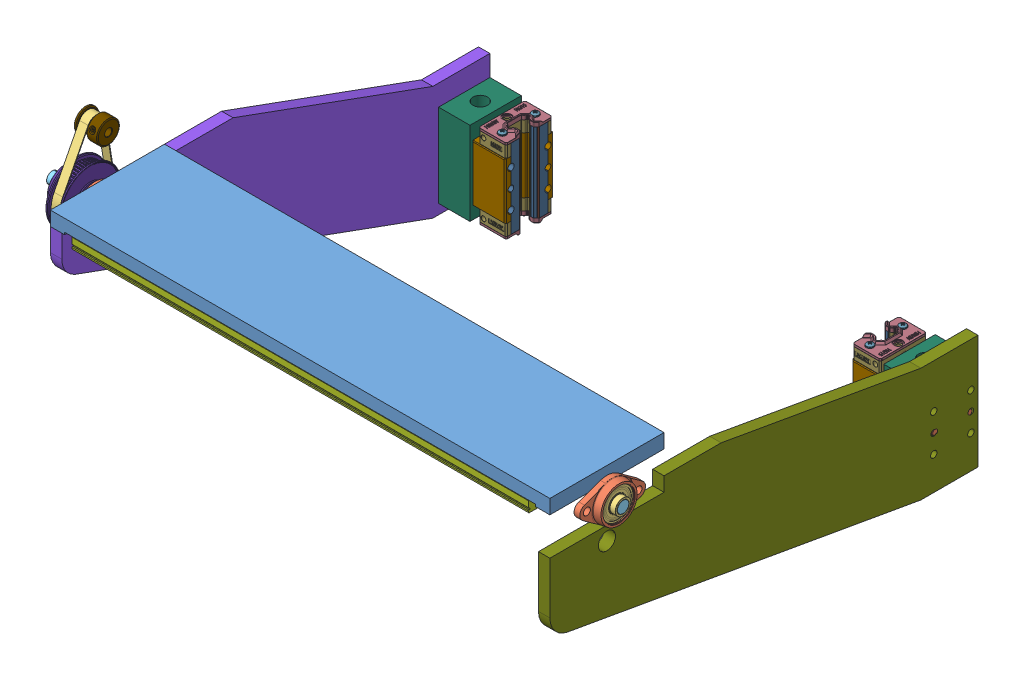
SolidWorks assembly Eje_X, configuration Predeterminado. Lengths in mm.
Overall size (400 162.38 300).
52 component instances, 22 part files, 43 mates.
Components (placement in the parent):
- Puente_X^Eje_X-1: Puente_X^Eje_X [Predeterminado] at (-189.2038 15.372 -72.2278) x (1 0 0) z (0 -1 0) size (350 80 10) (virtual)
- KFL08-1: KFL08 [Varsayılan] at (-189.2038 -4.128 -32.2278) x (0 -0.043192 0.999067) z (0 -0.999067 -0.043192) size (46.5 11.35 27)
  - FLANGE-1: FLANGE [Default] at origin size (46.5 8.5 27)
  - BEARING-1: BEARING [Default] at (0 4 0) x (1 0 0) z (0 -1 0) size (22 22 10.85)
  - socket set screw cone point_am-1: socket set screw cone point_am [B18.3.6M - M2.5 x 0.45 x 2 Hex Socket Cone Pt. SS --S] at (0 9.425 5.45) x (0 0 -1) z (1 0 0) size (2 2.5 2.5)
  - socket set screw cone point_am-2: socket set screw cone point_am [B18.3.6M - M2.5 x 0.45 x 2 Hex Socket Cone Pt. SS --S] at (5.45 9.425 0) x (-1 0 0) z (0 0 -1) size (2 2.5 2.5)
- ax_Y_LeadScrew_Nut_8mm_x_2mmPitch-1: ax_Y_LeadScrew_Nut_8mm_x_2mmPitch [Default] at (-227.8538 -4.128 -32.2278) x (0 0.538804 0.842431) z (-1 0 0) size (8 8 400)
- eje_X_guia_inf-1: eje_X_guia_inf [Predeterminado] at (75.7962 2.9226 -66.2278) x (0 0 -1) z (-1 0 0) size (12 8.1 320)
- eje_X_guia_sup-1: eje_X_guia_sup [Predeterminado] at (-104.2038 2.9226 1.7722) x (0 0 1) z (1 0 0) size (12 8.1 320)
-  Columa_xn^Eje_X-1:  Columa_xn^Eje_X [Predeterminado] at (-181.2038 -35.5839 -292.2278) x (0 -1 0) z (-1 0 0) size (130.96 300 8) (virtual)
- HGH15CA-1: HGH15CA [Default] at (-131.2038 -79.3839 -274.2278) x (0 0 -1) z (0 1 0) size (34 23.7 61.49)
  - HGH15CA Block-1: HGH15CA Block [HGR15R300CE20] at origin size (34 23.7 39.4)
  - HGx15CA Retainer-1: HGx15CA Retainer [HGR15R300CE20] at origin size (26 4 55.4)
  - HGx15CA Tiny Red-1: HGx15CA Tiny Red [HGR15R300CE20] at origin size (14.2 1 55.4)
  - HGx15CA End Cap-1: HGx15CA End Cap [HGR15R300CE20] at origin size (32.5 19.5 8)
  - HGx15CA End Cap-2: HGx15CA End Cap [HGR15R300CE20] x (-1 0 0) z (0 0 -1) size (32.5 19.5 8)
  - HGx15CA Seal-1: HGx15CA Seal [HGR15R300CE20] at origin size (32.5 19.5 3)
  - HGx15CA Seal-2: HGx15CA Seal [HGR15R300CE20] x (-1 0 0) z (0 0 -1) size (32.5 19.5 3)
  - pan head cross recess screw_iso-1: pan head cross recess screw_iso [ISO 7045 - M2.5 x 16 - Z - 16C] at (11.5 11.8 30.8) x (0 0 -1) z (0 -1 0) size (18.05 5 5)
  - pan head cross recess screw_iso-2: pan head cross recess screw_iso [ISO 7045 - M2.5 x 16 - Z - 16C] at (-11.5 11.8 30.8) x (0 0 -1) z (0 1 0) size (18.05 5 5)
  - pan head cross recess screw_iso-3: pan head cross recess screw_iso [ISO 7045 - M2.5 x 16 - Z - 16C] at (11.5 11.8 -30.8) x (0 0 1) z (0 -1 0) size (18.05 5 5)
  - pan head cross recess screw_iso-4: pan head cross recess screw_iso [ISO 7045 - M2.5 x 16 - Z - 16C] at (-11.5 11.8 -30.8) x (0 0 1) z (0 1 0) size (18.05 5 5)
- Soporte_tuerca_husillo_X^Eje_X-1: Soporte_tuerca_husillo_X^Eje_X [Predeterminado] at (-159.2038 -108.5839 -256.2278) x (0 1 0) z (-1 0 0) size (58.4 36 22) (virtual)
- Columa_xp^Eje_X-1: Columa_xp^Eje_X [Predeterminado] at (160.7962 -35.5839 -292.2278) x (0 -1 0) z (-1 0 0) size (130.96 300 8) (virtual)
- HGH15CA-2: HGH15CA [Default] at (102.7962 -79.3839 -274.2278) x (0 0 -1) z (0 -1 0) size (34 23.7 61.49)
  - HGH15CA Block-1: HGH15CA Block [HGR15R300CE20] at origin size (34 23.7 39.4)
  - HGx15CA Retainer-1: HGx15CA Retainer [HGR15R300CE20] at origin size (26 4 55.4)
  - HGx15CA Tiny Red-1: HGx15CA Tiny Red [HGR15R300CE20] at origin size (14.2 1 55.4)
  - HGx15CA End Cap-1: HGx15CA End Cap [HGR15R300CE20] at origin size (32.5 19.5 8)
  - HGx15CA End Cap-2: HGx15CA End Cap [HGR15R300CE20] x (-1 0 0) z (0 0 -1) size (32.5 19.5 8)
  - HGx15CA Seal-1: HGx15CA Seal [HGR15R300CE20] at origin size (32.5 19.5 3)
  - HGx15CA Seal-2: HGx15CA Seal [HGR15R300CE20] x (-1 0 0) z (0 0 -1) size (32.5 19.5 3)
  - pan head cross recess screw_iso-1: pan head cross recess screw_iso [ISO 7045 - M2.5 x 16 - Z - 16C] at (11.5 11.8 30.8) x (0 0 -1) z (0 -1 0) size (18.05 5 5)
  - pan head cross recess screw_iso-2: pan head cross recess screw_iso [ISO 7045 - M2.5 x 16 - Z - 16C] at (-11.5 11.8 30.8) x (0 0 -1) z (0 1 0) size (18.05 5 5)
  - pan head cross recess screw_iso-3: pan head cross recess screw_iso [ISO 7045 - M2.5 x 16 - Z - 16C] at (11.5 11.8 -30.8) x (0 0 1) z (0 -1 0) size (18.05 5 5)
  - pan head cross recess screw_iso-4: pan head cross recess screw_iso [ISO 7045 - M2.5 x 16 - Z - 16C] at (-11.5 11.8 -30.8) x (0 0 1) z (0 1 0) size (18.05 5 5)
- Soporte_tuerca_husillo_X^Eje_X-2: Soporte_tuerca_husillo_X^Eje_X [Predeterminado] at (130.7962 -50.1839 -256.2278) x (0 -1 0) z (1 0 0) size (58.4 36 22) (virtual)
- KFL08-2: KFL08 [Varsayılan] at (160.7962 -4.128 -32.2278) x (0 -0.14239 -0.989811) z (0 -0.989811 0.14239) size (46.5 11.35 27)
  - FLANGE-1: FLANGE [Default] at origin size (46.5 8.5 27)
  - BEARING-1: BEARING [Default] at (0 4 0) x (1 0 0) z (0 -1 0) size (22 22 10.85)
  - socket set screw cone point_am-1: socket set screw cone point_am [B18.3.6M - M2.5 x 0.45 x 2 Hex Socket Cone Pt. SS --S] at (0 9.425 5.45) x (0 0 -1) z (1 0 0) size (2 2.5 2.5)
  - socket set screw cone point_am-2: socket set screw cone point_am [B18.3.6M - M2.5 x 0.45 x 2 Hex Socket Cone Pt. SS --S] at (5.45 9.425 0) x (-1 0 0) z (0 0 -1) size (2 2.5 2.5)
- Copia de GT2_60T_8_6^Eje_X-1: Copia de GT2_60T_8_6^Eje_X [Default] at (-211.3538 -4.128 -32.2278) x (0 -0.85392 -0.520404) z (1 0 0) size (42 42 18) (virtual)
- Copia de GT2_20T^Eje_X-1: Copia de GT2_20T^Eje_X [Конфигурация1] at (-194.9038 36.3557 -38.7137) x (-1 0 0) z (0 0.380598 0.924741) size (16 16 16) (virtual)
- Copia de NEMA 23HS7430^Eje_X-1: Copia de NEMA 23HS7430^Eje_X [По умолчанию] at (-187.6038 45.572 -50.4278) x (0 1 0) z (1 0 0) size (58.4 56.4 95.6) (hidden, virtual)
- Copia de T8_nut^Eje_X-1: Copia de T8_nut^Eje_X [Default] at (-170.2038 -112.5839 -274.4641) x (0.063591 0 0.997976) z (-0.997976 0 0.063591) size (22.03 15.25 22.03) (virtual)
- Copia de T8_nut^Eje_X-2: Copia de T8_nut^Eje_X [Default] at (141.7962 -112.5839 -274.4641) x (0.864495 0 0.502641) z (-0.502641 0 0.864495) size (22.03 15.25 22.03) (virtual)
- guia_4x20^Eje_X-1: guia_4x20^Eje_X [Predeterminado] at (-169.2038 -79.3839 -262.2278) x (0 0 1) z (-1 0 0) size (4 4 20) (virtual)
- guia_4x20^Eje_X-2: guia_4x20^Eje_X [Predeterminado] at (-169.2038 -79.3839 -286.2278) x (0 0 1) z (-1 0 0) size (4 4 20) (virtual)
- Correa_158^Eje_X-1: Correa_158^Eje_X [Predeterminado] at (-209.3538 -4.128 -32.2278) x (0 0.987408 -0.158192) z (1 0 0) size (66.95 38.7 6) (virtual)
- guia_4x20^Eje_X-3: guia_4x20^Eje_X [Predeterminado] at (140.7962 -79.3839 -262.2278) x (0 -0.924225 -0.381849) z (1 0 0) size (4 4 20) (virtual)
- guia_4x20^Eje_X-4: guia_4x20^Eje_X [Predeterminado] at (140.7962 -79.3839 -286.2278) x (0 -0.305624 0.952152) z (1 0 0) size (4 4 20) (virtual)
Mates (geometry in assembly coordinates):
- Coincidente8: coincident aligned: plane of Puente_X^Eje_X-1 through (-189.2038 5.372 7.7722) normal (-1 0 0); plane of  Columa_xn^Eje_X-1 through (-189.2038 -10.4485 -7.2278) normal (-1 0 0)
- Coincidente9: coincident anti-aligned: plane of Puente_X^Eje_X-1 through (-189.2038 5.372 -72.2278) normal (0 -1 0); plane of  Columa_xn^Eje_X-1 through (-189.2038 5.372 7.7722) normal (0 1 0)
- Coincidente10: coincident anti-aligned: plane of Puente_X^Eje_X-1 through (160.7962 5.372 -72.2278) normal (0 0 -1); plane of  Columa_xn^Eje_X-1 through (-189.2038 15.372 -72.2278) normal (0 0 1)
- Coincidente11: coincident aligned: plane of Puente_X^Eje_X-1 through (160.7962 5.372 7.7722) normal (1 0 0); plane of Columa_xp^Eje_X-1 through (160.7962 -10.4485 -7.2278) normal (1 0 0)
- Coincidente12: coincident anti-aligned: plane of Puente_X^Eje_X-1 through (160.7962 5.372 -72.2278) normal (0 0 -1); plane of Columa_xp^Eje_X-1 through (152.7962 15.372 -72.2278) normal (0 0 1)
- Coincidente13: coincident anti-aligned: plane of Puente_X^Eje_X-1 through (-189.2038 5.372 -72.2278) normal (0 -1 0); plane of Columa_xp^Eje_X-1 through (152.7962 5.372 7.7722) normal (0 1 0)
- Coincidente16: coincident aligned: plane of Puente_X^Eje_X-1 through (160.7962 5.372 7.7722) normal (0 0 1); plane of eje_X_guia_sup-1 through (145.7962 6.872 7.7722) normal (0 0 1)
- Coincidente20: coincident anti-aligned: plane of KFL08-1/FLANGE-1 through (-189.2038 -4.9163 -13.9949) normal (1 0 0); plane of  Columa_xn^Eje_X-1 through (-189.2038 -10.4485 -7.2278) normal (-1 0 0)
- Concéntrica2: concentric anti-aligned: cylinder of KFL08-1/BEARING-1 through (-189.7038 -4.128 -32.2278) axis (1 0 0) radius 4; cylinder of ax_Y_LeadScrew_Nut_8mm_x_2mmPitch-1 through (172.1462 -4.128 -32.2278) axis (-1 0 0) radius 4
- Coincidente28: coincident anti-aligned: plane of Columa_xp^Eje_X-1 through (160.7962 -10.4485 -7.2278) normal (1 0 0); plane of KFL08-2/FLANGE-1 through (160.7962 -6.7267 -50.2919) normal (-1 0 0)
- Concéntrica3: concentric aligned: cylinder of ax_Y_LeadScrew_Nut_8mm_x_2mmPitch-1 through (172.1462 -4.128 -32.2278) axis (-1 0 0) radius 4; cylinder of KFL08-2/BEARING-1 through (161.2962 -4.128 -32.2278) axis (-1 0 0) radius 4
- Coincidente29: coincident aligned: plane of ax_Y_LeadScrew_Nut_8mm_x_2mmPitch-1 through (172.1462 -4.128 -32.2278) normal (1 0 0); plane of KFL08-2/BEARING-1 through (172.1462 -8.3842 -31.6155) normal (1 0 0)
- Concéntrica4: concentric aligned: cylinder of ax_Y_LeadScrew_Nut_8mm_x_2mmPitch-1 through (172.1462 -4.128 -32.2278) axis (-1 0 0) radius 4; cylinder of Copia de GT2_60T_8_6^Eje_X-1 through (-181.3538 -4.128 -32.2278) axis (-1 0 0) radius 4
- Distancia3: distance = 9 mm aligned: plane of Copia de GT2_60T_8_6^Eje_X-1 through (-218.8538 -4.128 -32.2278) normal (-1 0 0); plane of ax_Y_LeadScrew_Nut_8mm_x_2mmPitch-1 through (-227.8538 -4.128 -32.2278) normal (-1 0 0)
- Coincidente32: coincident aligned: plane of Puente_X^Eje_X-1 through (160.7962 5.372 -72.2278) normal (0 0 -1); plane of eje_X_guia_inf-1 through (-174.2038 6.872 -72.2278) normal (0 0 -1)
- Concéntrica6: concentric anti-aligned: cylinder of ax_Y_LeadScrew_Nut_8mm_x_2mmPitch-1 through (172.1462 -4.128 -32.2278) axis (-1 0 0) radius 4; cylinder of  Columa_xn^Eje_X-1 through (-189.2038 -4.128 -32.2278) axis (1 0 0) radius 6
- Coincidente33: coincident aligned: plane of Puente_X^Eje_X-1 through (-189.2038 5.372 7.7722) normal (-1 0 0); plane of Copia de NEMA 23HS7430^Eje_X-1 through (-189.2038 45.572 -50.4278) normal (-1 0 0)
- Distancia6: distance = 2 mm anti-aligned: plane of Copia de NEMA 23HS7430^Eje_X-1 through (-177.6038 17.372 -78.6278) normal (0 -1 0); plane of Puente_X^Eje_X-1 through (-189.2038 15.372 -72.2278) normal (0 1 0)
- Distancia7: distance = 30 mm aligned: plane of Copia de NEMA 23HS7430^Eje_X-1 through (-177.6038 17.372 -22.2278) normal (0 0 1); plane of Puente_X^Eje_X-1 through (160.7962 5.372 7.7722) normal (0 0 1)
- Coincidente42: coincident anti-aligned: plane of  Columa_xn^Eje_X-1 through (-181.2038 -10.4485 -7.2278) normal (1 0 0); plane of Soporte_tuerca_husillo_X^Eje_X-1 through (-181.2038 -108.5839 -256.2278) normal (-1 0 0)
- Distancia10: distance = 7 mm aligned: plane of Soporte_tuerca_husillo_X^Eje_X-1 through (-181.2038 -108.5839 -256.2278) normal (0 -1 0); plane of  Columa_xn^Eje_X-1 through (-189.2038 -115.5839 -292.2278) normal (0 -1 0)
- Coincidente44: coincident aligned: plane of  Columa_xn^Eje_X-1 through (-189.2038 -35.5839 -292.2278) normal (0 0 -1); plane of Soporte_tuerca_husillo_X^Eje_X-1 through (-181.2038 -108.5839 -292.2278) normal (0 0 -1)
- Coincidente45: coincident anti-aligned: plane of HGH15CA-1/HGH15CA Block-1 through (-159.2038 -59.6839 -290.2278) normal (-1 0 0); plane of Soporte_tuerca_husillo_X^Eje_X-1 through (-159.2038 -108.5839 -256.2278) normal (1 0 0)
- Distancia11: distance = 1 mm aligned: plane of HGH15CA-1/HGH15CA Block-1 through (-136.5038 -59.6839 -291.2278) normal (0 0 -1); plane of Soporte_tuerca_husillo_X^Eje_X-1 through (-181.2038 -108.5839 -292.2278) normal (0 0 -1)
- Coincidente47: coincident aligned: plane of HGH15CA-1/HGx15CA Seal-2 through (-137.6195 -108.5839 -279.3778) normal (0 -1 0); plane of Soporte_tuerca_husillo_X^Eje_X-1 through (-181.2038 -108.5839 -256.2278) normal (0 -1 0)
- Concéntrica7: concentric anti-aligned: cylinder of  Columa_xn^Eje_X-1 through (-189.2038 -79.3839 -262.2278) axis (-1 0 0) radius 2; cylinder of guia_4x20^Eje_X-1 through (-189.2038 -79.3839 -262.2278) axis (1 0 0) radius 2
- Coincidente48: coincident aligned: plane of  Columa_xn^Eje_X-1 through (-189.2038 -10.4485 -7.2278) normal (-1 0 0); plane of guia_4x20^Eje_X-1 through (-189.2038 -79.3839 -262.2278) normal (-1 0 0)
- Coincidente49: coincident aligned: plane of  Columa_xn^Eje_X-1 through (-189.2038 -10.4485 -7.2278) normal (-1 0 0); plane of guia_4x20^Eje_X-2 through (-189.2038 -79.3839 -286.2278) normal (-1 0 0)
- Concéntrica8: concentric anti-aligned: cylinder of  Columa_xn^Eje_X-1 through (-189.2038 -79.3839 -286.2278) axis (-1 0 0) radius 2; cylinder of guia_4x20^Eje_X-2 through (-189.2038 -79.3839 -286.2278) axis (1 0 0) radius 2
- Concéntrica9: concentric anti-aligned: cylinder of Correa_158^Eje_X-1 through (-203.3538 -4.128 -32.2278) axis (-1 0 0) radius 18.85; cylinder of Copia de GT2_60T_8_6^Eje_X-1 through (-218.8538 -4.128 -32.2278) axis (1 0 0) radius 12.5
- Distancia12: distance = 1 mm anti-aligned: plane of Correa_158^Eje_X-1 through (-203.3538 -4.128 -32.2278) normal (1 0 0); plane of Copia de GT2_60T_8_6^Eje_X-1 through (-202.3538 -4.128 -32.2278) normal (-1 0 0)
- Concéntrica10: concentric anti-aligned: cylinder of Copia de GT2_20T^Eje_X-1 through (-194.9038 36.3557 -38.7137) axis (1 0 0) radius 8; cylinder of Correa_158^Eje_X-1 through (-203.3538 36.3557 -38.7137) axis (-1 0 0) radius 6.1
- Distancia13: distance = 1 mm anti-aligned: plane of Correa_158^Eje_X-1 through (-203.3538 -4.128 -32.2278) normal (1 0 0); plane of Copia de GT2_20T^Eje_X-1 through (-202.3538 36.3557 -38.7137) normal (-1 0 0)
- Coincidente50: coincident anti-aligned: plane of Columa_xp^Eje_X-1 through (152.7962 -10.4485 -7.2278) normal (-1 0 0); plane of Soporte_tuerca_husillo_X^Eje_X-2 through (152.7962 -50.1839 -256.2278) normal (1 0 0)
- Coincidente51: coincident aligned: plane of Columa_xp^Eje_X-1 through (152.7962 -35.5839 -292.2278) normal (0 0 -1); plane of Soporte_tuerca_husillo_X^Eje_X-2 through (152.7962 -50.1839 -292.2278) normal (0 0 -1)
- Distancia14: distance = 7 mm aligned: plane of Soporte_tuerca_husillo_X^Eje_X-2 through (152.7962 -108.5839 -256.2278) normal (0 -1 0); plane of Columa_xp^Eje_X-1 through (152.7962 -115.5839 -292.2278) normal (0 -1 0)
- Coincidente53: coincident anti-aligned: circle of Soporte_tuerca_husillo_X^Eje_X-2; circle of Copia de T8_nut^Eje_X-2
- Distancia15: distance = 1 mm aligned: plane of HGH15CA-2/HGH15CA Block-1 through (108.0962 -99.0839 -291.2278) normal (0 0 -1); plane of Soporte_tuerca_husillo_X^Eje_X-2 through (152.7962 -50.1839 -292.2278) normal (0 0 -1)
- Coincidente55: coincident aligned: plane of HGH15CA-2/HGx15CA Seal-1 through (109.2119 -108.5839 -269.0778) normal (0 -1 0); plane of Soporte_tuerca_husillo_X^Eje_X-2 through (152.7962 -108.5839 -256.2278) normal (0 -1 0)
- Coincidente56: coincident aligned: plane of Columa_xp^Eje_X-1 through (160.7962 -10.4485 -7.2278) normal (1 0 0); plane of guia_4x20^Eje_X-3 through (160.7962 -79.3839 -262.2278) normal (1 0 0)
- Concéntrica11: concentric aligned: circle of Columa_xp^Eje_X-1; circle of guia_4x20^Eje_X-4
- Concéntrica12: concentric anti-aligned: cylinder of Columa_xp^Eje_X-1 through (160.7962 -79.3839 -262.2278) axis (1 0 0) radius 2; cylinder of guia_4x20^Eje_X-3 through (160.7962 -79.3839 -262.2278) axis (-1 0 0) radius 2
- Coincidente57: coincident aligned: plane of Columa_xp^Eje_X-1 through (160.7962 -10.4485 -7.2278) normal (1 0 0); plane of guia_4x20^Eje_X-4 through (160.7962 -79.3839 -286.2278) normal (1 0 0)
